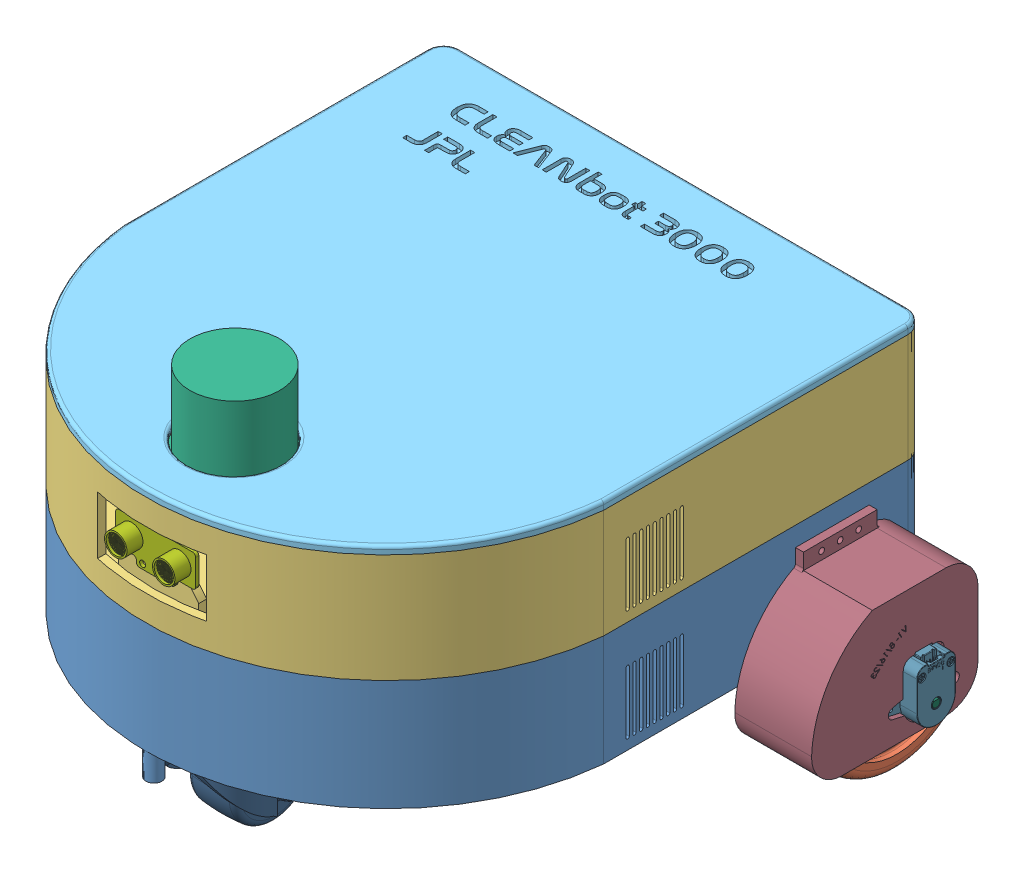
SolidWorks assembly Cleanbot_V2, configuration Default. Lengths in mm.
Overall size (522.89 339.19 460.61).
18 component instances, 15 part files, 33 mates.
Components (placement in the parent):
- Chassis2(level1)-1: Chassis2(level1) [Default] at (23.4837 42.2412 -178.9478) size (381 108.78 426.72)
- Back wheels-2: Back wheels [Default] at (-206.6183 23.0642 -331.3478) x (1 0 0) z (0 -0.725001 -0.688748) size (30.48 127 127)
- Chassis2(level2)-1: Chassis2(level2) [Default] at (23.4837 130.2412 -178.9478) size (381 121.92 426.72)
- ZyboB-1: ZyboB [Default] at (-70.4963 144.2112 -266.5778) size (124.46 58.42 177.8)
- Chassis2(cover)-1: Chassis2(cover) [Default] at (23.4837 216.6012 -178.9478) size (381 22.86 426.72)
- LiDAR-1: LiDAR [Default] at (23.4837 165.8012 -56.1696) x (-1 0 0) z (0 0 -1) size (76.2 104.14 114.3)
- Sonar-1: Sonar [Default] at (23.5949 174.0562 24.2522) size (63.5 31.75 15.24)
- BLWRPG093S-R139.step-2: BLWRPG093S-R139.step [Default] at (-121.7663 23.0642 -331.3478) x (0 0.086499 -0.996252) z (-1 0 0) size (22.09 22.09 182.75)
- channel15-1: channel15 [Default] at (-167.0163 4.1412 -312.2978) x (0 0 -1) z (1 0 0) size (38.1 38.1 381)
- Back wheels-3: Back wheels [Default] at (253.5857 23.0642 -331.3478) x (-1 0 0) z (0 0.725001 0.688748) size (30.48 127 127)
- BLWRPG093S-R139.step-3: BLWRPG093S-R139.step [Default] at (168.7337 23.0642 -331.3478) x (0 -0.086499 0.996252) z (1 0 0) size (22.09 22.09 182.75)
- Caster-1: Caster [Default] at (23.4837 -40.1588 -26.7787) x (-1 0 0) z (0 0 -1) size (90 92 99.5)
- encoderHolder-1: encoderHolder [Default] at (-179.7163 51.4035 -308.3229) x (0 0 -1) z (0 1 0) size (132.05 60.96 114.3)
- ENC-A5SX-XXXX-250-H-G-2: ENC-A5SX-XXXX-250-H-G [Default] at (-221.3723 23.0642 -331.3478) x (0 0 -1) z (-1 0 0) size (53.71 47.11 16.59)
- MirrorencoderHolder-3: MirrorencoderHolder [Default] at (226.6837 51.4035 -308.3229) x (0 0 -1) z (0 -1 0) size (132.05 60.96 114.3)
- MirrorENC-A5SX-XXXX-250-H-G-5: MirrorENC-A5SX-XXXX-250-H-G [Default] at (268.3397 23.0642 -331.3478) x (0 0 -1) z (-1 0 0) size (53.71 47.11 16.59)
- shaftextendr-2: shaftextendr [Default] at (-204.6083 23.0642 -331.3478) x (0 -0.999684 -0.025149) z (-1 0 0) size (12.7 12.7 33.35)
- shaftextendr-3: shaftextendr [Default] at (251.5757 23.0642 -331.3478) x (0 0.999684 0.025149) z (1 0 0) size (12.7 12.7 33.35)
Mates (geometry in assembly coordinates):
- Coincident30: coincident anti-aligned: circle of Chassis2(level1)-1; cylinder of Chassis2(level2)-1 through (-154.3163 220.4112 -138.6212) axis (0 -1 0) radius 3.175
- Coincident35: coincident anti-aligned: plane of Chassis2(level2)-1 through (23.4837 144.2112 -178.9478) normal (0 1 0); plane of ZyboB-1 through (-70.4963 144.2112 -266.5778) normal (0 -1 0)
- Concentric5: concentric anti-aligned: cylinder of Chassis2(level2)-1 through (201.2837 220.4112 -379.6078) axis (0 -1 0) radius 3.175; cylinder of Chassis2(cover)-1 through (201.2837 200.0912 -379.6078) axis (0 1 0) radius 3.175
- Coincident37: coincident aligned: circle of Chassis2(level2)-1; circle of Chassis2(cover)-1
- Coincident39: coincident aligned: circle of Chassis2(level1)-1; circle of Chassis2(level2)-1
- Concentric82: concentric anti-aligned: cylinder of Chassis2(level2)-1 through (-126.3763 144.2112 -349.1278) axis (0 -1 0) radius 2.54; cylinder of ZyboB-1 through (-126.3763 136.5912 -349.1278) axis (0 1 0) radius 2.54
- Concentric83: concentric anti-aligned: cylinder of Chassis2(level2)-1 through (-126.3763 144.2112 -184.0278) axis (0 -1 0) radius 2.54; cylinder of ZyboB-1 through (-126.3763 136.5912 -184.0278) axis (0 1 0) radius 2.54
- Concentric85: concentric anti-aligned: cylinder of Chassis2(level2)-1 through (55.2337 168.3412 -5.7198) axis (0 -1 0) radius 2.54; cylinder of LiDAR-1 through (55.2337 168.3412 -5.7198) axis (0 1 0) radius 2.54
- Coincident497: coincident aligned: circle of Chassis2(level2)-1; cylinder of LiDAR-1 through (-8.2663 168.3412 -5.7198) axis (0 1 0) radius 2.54
- Coincident498: coincident anti-aligned: plane of Chassis2(level2)-1 through (23.4837 168.3412 -178.9478) normal (0 1 0); plane of LiDAR-1 through (23.4837 168.3412 -56.1696) normal (0 -1 0)
- Coincident501: coincident anti-aligned: plane of Chassis2(level2)-1 through (-8.2663 172.1512 24.2522) normal (0 0 1); plane of Sonar-1 through (23.5949 174.0562 24.2522) normal (0 0 -1)
- Concentric86: concentric aligned: circle of Chassis2(level2)-1; circle of Sonar-1
- Concentric87: concentric aligned: circle of Chassis2(level2)-1; circle of Sonar-1
- Coincident509: coincident anti-aligned: plane of Chassis2(level1)-1 through (23.4837 42.2412 -178.9478) normal (0 -1 0); plane of channel15-1 through (213.9837 42.2412 -312.2978) normal (0 1 0)
- Parallel2: parallel anti-aligned: line of Chassis2(level1)-1 through (-154.3163 42.2412 -392.3078) axis (1 0 0); line of channel15-1 through (211.4437 42.2412 -350.3978) axis (-1 0 0)
- Coincident510: coincident aligned: plane of Chassis2(level1)-1 through (213.9837 130.2412 -178.9478) normal (1 0 0); plane of channel15-1 through (213.9837 4.1412 -312.2978) normal (1 0 0)
- Distance2: distance = 41.91 mm aligned: plane of channel15-1 through (213.9837 42.2412 -350.3978) normal (0 0 -1); plane of Chassis2(level1)-1 through (23.4837 130.2412 -392.3078) normal (0 0 -1)
- Concentric90: concentric anti-aligned: circle of Back wheels-2; cylinder of BLWRPG093S-R139.step-2 through (-184.2663 23.0642 -331.3478) axis (1 0 0) radius 3
- Concentric91: concentric anti-aligned: cylinder of BLWRPG093S-R139.step-2 through (-53.7663 23.0642 -331.3478) axis (-1 0 0) radius 11; circle of channel15-1
- Distance6: distance = 17.272 mm aligned: plane of Back wheels-2 through (-201.5383 23.0642 -331.3478) normal (-1 0 0); plane of BLWRPG093S-R139.step-2 through (-184.2663 23.0642 -331.3478) normal (-1 0 0)
- Coincident516: coincident aligned: plane of BLWRPG093S-R139.step-2 through (-167.0163 23.0642 -331.3478) normal (-1 0 0); plane of channel15-1 through (-167.0163 4.1412 -312.2978) normal (-1 0 0)
- Parallel3: parallel aligned: plane of channel15-1 through (213.9837 4.1412 -312.2978) normal (0 0 1); plane of Caster-1 through (58.4837 47.8412 18.2213) normal (0 0 1)
- Parallel4: parallel aligned: plane of Chassis2(level1)-1 through (213.9837 130.2412 -178.9478) normal (1 0 0); plane of Caster-1 through (68.4837 47.8412 8.2213) normal (1 0 0)
- Coincident518: coincident aligned: plane of Chassis2(level1)-1 through (23.4837 42.2412 -178.9478) normal (0 -1 0); plane of Caster-1 through (23.4837 42.2412 6.7213) normal (0 -1 0)
- Concentric92: concentric aligned: circle of Chassis2(level1)-1; circle of Caster-1
- Coincident522: coincident anti-aligned: plane of encoderHolder-1 through (-221.3723 23.0642 -355.5108) normal (-1 0 0); plane of ENC-A5SX-XXXX-250-H-G-2 through (-221.3723 23.0642 -331.3478) normal (1 0 0)
- Concentric95: concentric anti-aligned: cylinder of Back wheels-2 through (-220.6275 23.0642 -331.3478) axis (1 0 0) radius 4.953; cylinder of encoderHolder-1 through (-179.7163 23.0642 -331.3478) axis (-1 0 0) radius 8.001
- Parallel7: parallel aligned: plane of Chassis2(level1)-1 through (23.4837 130.2412 -392.3078) normal (0 0 -1); plane of encoderHolder-1 through (-227.9763 0.6035 -374.3629) normal (0 0 -1)
- Concentric97: concentric anti-aligned: cylinder of encoderHolder-1 through (-179.7163 23.0642 -331.3478) axis (-1 0 0) radius 8.001; cylinder of ENC-A5SX-XXXX-250-H-G-2 through (-225.8681 23.0642 -331.3478) axis (1 0 0) radius 3.1763
- Concentric98: concentric anti-aligned: cylinder of encoderHolder-1 through (-179.7163 23.0642 -354.3602) axis (-1 0 0) radius 1.651; cylinder of ENC-A5SX-XXXX-250-H-G-2 through (-241.7432 23.0642 -354.3602) axis (1 0 0) radius 1.3843
- Coincident524: coincident anti-aligned: plane of Chassis2(level1)-1 through (-167.0163 130.2412 -178.9478) normal (-1 0 0); plane of encoderHolder-1 through (-167.0163 23.0642 -331.3478) normal (1 0 0)
- Concentric101: concentric aligned: cylinder of ENC-A5SX-XXXX-250-H-G-2 through (-225.8681 23.0642 -331.3478) axis (1 0 0) radius 3.1763; cylinder of shaftextendr-2 through (-237.9585 23.0642 -331.3478) axis (1 0 0) radius 3.048
- Coincident526: coincident aligned: plane of ENC-A5SX-XXXX-250-H-G-2 through (-237.9585 23.0642 -331.3478) normal (-1 0 0); plane of shaftextendr-2 through (-237.9585 23.0642 -331.3478) normal (-1 0 0)
